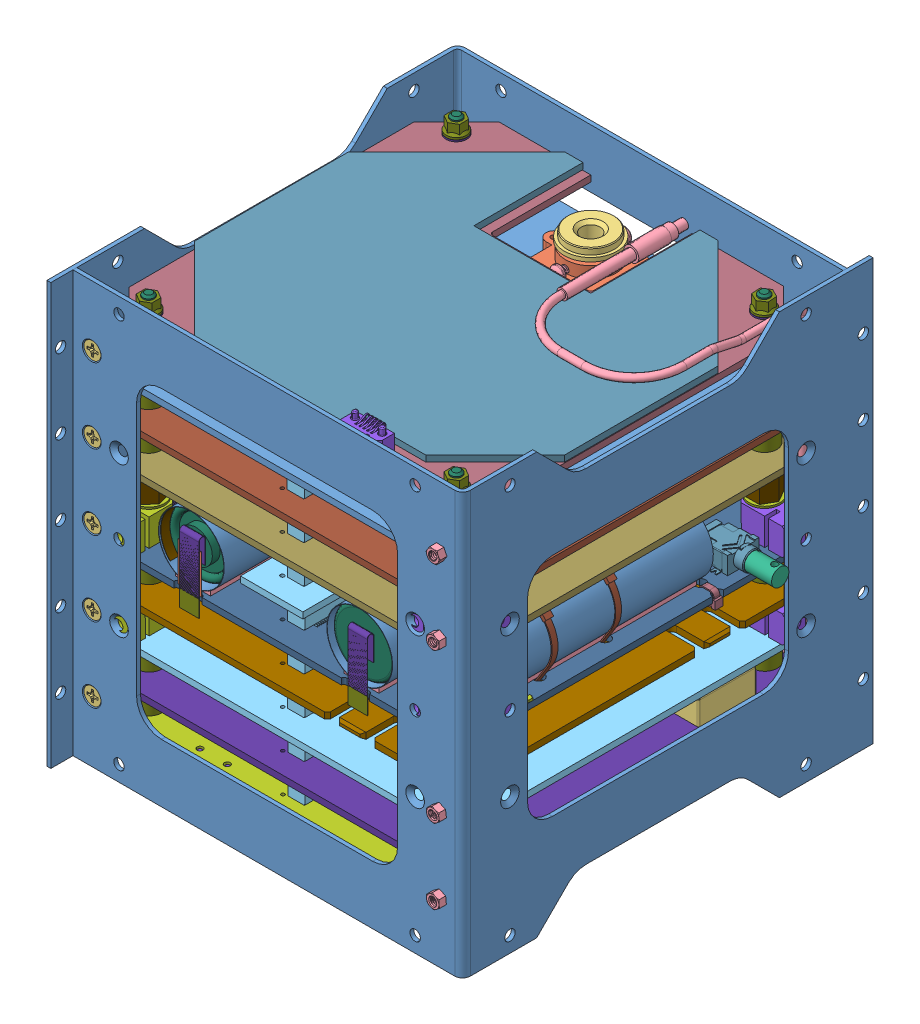
SolidWorks assembly FOX_FrameAssembly, configuration Default. Lengths in mm.
Overall size (104.5 108 111.03).
292 component instances, 63 part files, 95 mates.
Components (placement in the parent):
- FOX_ME_111_Walls-1: FOX_ME_111_Walls [Default] at (75.0611 9.8692 29.0204) size (100.17 108 105.36)
- FOX_ME_111_Walls-2: FOX_ME_111_Walls [Default] at (-24.2839 9.8692 -70.6584) x (-1 0 0) z (0 0 -1) size (100.17 108 105.36)
- 90945A705_18-8 Stainless Steel Mil. Spec. Washer-1: 90945A705_18-8 Stainless Steel Mil. Spec. Washer [90945A705] at (70.0611 -28.5308 28.0204) x (1 0 0) z (0 -1 0) size (3.78 0.46 3.78)
- 90945A705_18-8 Stainless Steel Mil. Spec. Washer-2: 90945A705_18-8 Stainless Steel Mil. Spec. Washer [90945A705] at (-19.2839 -28.5308 -69.6584) x (1 0 0) z (0 1 0) size (3.78 0.46 3.78)
- 90945A705_18-8 Stainless Steel Mil. Spec. Washer-3: 90945A705_18-8 Stainless Steel Mil. Spec. Washer [90945A705] at (-19.2839 29.0692 -69.6584) x (1 0 0) z (0 1 0) size (3.78 0.46 3.78)
- 90945A705_18-8 Stainless Steel Mil. Spec. Washer-4: 90945A705_18-8 Stainless Steel Mil. Spec. Washer [90945A705] at (-19.2839 -9.3308 -69.6584) x (1 0 0) z (0 1 0) size (3.78 0.46 3.78)
- 90945A705_18-8 Stainless Steel Mil. Spec. Washer-5: 90945A705_18-8 Stainless Steel Mil. Spec. Washer [90945A705] at (70.0611 9.8692 -68.6584) x (1 0 0) z (0 -1 0) size (3.78 0.46 3.78)
- 90945A705_18-8 Stainless Steel Mil. Spec. Washer-6: 90945A705_18-8 Stainless Steel Mil. Spec. Washer [90945A705] at (-19.2839 9.8692 -69.6584) x (1 0 0) z (0 1 0) size (3.78 0.46 3.78)
- 90945A705_18-8 Stainless Steel Mil. Spec. Washer-7: 90945A705_18-8 Stainless Steel Mil. Spec. Washer [90945A705] at (70.0611 -9.3308 28.0204) x (1 0 0) z (0 -1 0) size (3.78 0.46 3.78)
- 90945A705_18-8 Stainless Steel Mil. Spec. Washer-8: 90945A705_18-8 Stainless Steel Mil. Spec. Washer [90945A705] at (70.0611 48.2692 28.0204) x (1 0 0) z (0 -1 0) size (3.78 0.46 3.78)
- 90945A705_18-8 Stainless Steel Mil. Spec. Washer-9: 90945A705_18-8 Stainless Steel Mil. Spec. Washer [90945A705] at (70.0611 29.0692 28.0204) x (1 0 0) z (0 -1 0) size (3.78 0.46 3.78)
- 90945A705_18-8 Stainless Steel Mil. Spec. Washer-20: 90945A705_18-8 Stainless Steel Mil. Spec. Washer [90945A705] at (-19.2839 48.2692 -70.1156) x (1 0 0) z (0 -1 0) size (3.78 0.46 3.78)
- 93085A017_Mil. Spec. Stainless Steel Phillips Flat Head Screws-1: 93085A017_Mil. Spec. Stainless Steel Phillips Flat Head Screws [93085A017] at (-19.2839 9.8692 25.6645) size (4.37 4.37 6.55)
- 93085A017_Mil. Spec. Stainless Steel Phillips Flat Head Screws-2: 93085A017_Mil. Spec. Stainless Steel Phillips Flat Head Screws [93085A017] at (-19.2839 48.2692 25.6645) size (4.37 4.37 6.55)
- 93085A017_Mil. Spec. Stainless Steel Phillips Flat Head Screws-3: 93085A017_Mil. Spec. Stainless Steel Phillips Flat Head Screws [93085A017] at (-19.2839 -9.3308 25.6645) size (4.37 4.37 6.55)
- 93085A017_Mil. Spec. Stainless Steel Phillips Flat Head Screws-4: 93085A017_Mil. Spec. Stainless Steel Phillips Flat Head Screws [93085A017] at (-19.2839 -28.5308 25.6645) size (4.37 4.37 6.55)
- 93085A017_Mil. Spec. Stainless Steel Phillips Flat Head Screws-5: 93085A017_Mil. Spec. Stainless Steel Phillips Flat Head Screws [93085A017] at (-19.2839 29.0692 25.6645) size (4.37 4.37 6.55)
- 93085A017_Mil. Spec. Stainless Steel Phillips Flat Head Screws-6: 93085A017_Mil. Spec. Stainless Steel Phillips Flat Head Screws [93085A017] at (70.0611 -28.5308 -67.3025) x (1 0 0) z (0 0 -1) size (4.37 4.37 6.55)
- 93085A017_Mil. Spec. Stainless Steel Phillips Flat Head Screws-7: 93085A017_Mil. Spec. Stainless Steel Phillips Flat Head Screws [93085A017] at (70.0611 -9.3308 -67.3025) x (1 0 0) z (0 0 -1) size (4.37 4.37 6.55)
- 93085A017_Mil. Spec. Stainless Steel Phillips Flat Head Screws-8: 93085A017_Mil. Spec. Stainless Steel Phillips Flat Head Screws [93085A017] at (70.0611 9.8692 -67.3025) x (1 0 0) z (0 0 -1) size (4.37 4.37 6.55)
- 93085A017_Mil. Spec. Stainless Steel Phillips Flat Head Screws-9: 93085A017_Mil. Spec. Stainless Steel Phillips Flat Head Screws [93085A017] at (70.0611 29.0692 -67.3025) x (1 0 0) z (0 0 -1) size (4.37 4.37 6.55)
- 93085A017_Mil. Spec. Stainless Steel Phillips Flat Head Screws-10: 93085A017_Mil. Spec. Stainless Steel Phillips Flat Head Screws [93085A017] at (70.0611 48.2692 -67.3025) x (-1 0 0) z (0 0 -1) size (4.37 4.37 6.55)
- 95307A800_Mil. Spec. Distorted-Thread Flange Locknut-1: 95307A800_Mil. Spec. Distorted-Thread Flange Locknut [95307A800] at (70.0611 -9.3308 29.6682) x (0.377464 0.926024 0) z (0 0 1) size (4.24 4.24 2.44)
- 95307A800_Mil. Spec. Distorted-Thread Flange Locknut-2: 95307A800_Mil. Spec. Distorted-Thread Flange Locknut [95307A800] at (70.0611 48.2692 29.6682) x (-0.835302 0.549792 0) z (0 0 1) size (4.24 4.24 2.44)
- 95307A800_Mil. Spec. Distorted-Thread Flange Locknut-3: 95307A800_Mil. Spec. Distorted-Thread Flange Locknut [95307A800] at (70.0611 29.0692 29.6682) x (0.533227 -0.845972 0) z (0 0 1) size (4.24 4.24 2.44)
- 95307A800_Mil. Spec. Distorted-Thread Flange Locknut-4: 95307A800_Mil. Spec. Distorted-Thread Flange Locknut [95307A800] at (70.0611 9.8692 -67.0106) x (-0.854944 -0.518721 0) z (0 0 1) size (4.24 4.24 2.44)
- 95307A800_Mil. Spec. Distorted-Thread Flange Locknut-5: 95307A800_Mil. Spec. Distorted-Thread Flange Locknut [95307A800] at (70.0611 -28.5308 29.6682) x (0.994964 0.100237 0) z (0 0 1) size (4.24 4.24 2.44)
- 95307A800_Mil. Spec. Distorted-Thread Flange Locknut-6: 95307A800_Mil. Spec. Distorted-Thread Flange Locknut [95307A800] at (-19.2839 48.2692 -71.3063) x (-0.82039 0.571804 0) z (0 0 -1) size (4.24 4.24 2.44)
- 95307A800_Mil. Spec. Distorted-Thread Flange Locknut-7: 95307A800_Mil. Spec. Distorted-Thread Flange Locknut [95307A800] at (-19.2839 29.0692 -71.3063) x (-0.204746 -0.978815 0) z (0 0 -1) size (4.24 4.24 2.44)
- 95307A800_Mil. Spec. Distorted-Thread Flange Locknut-8: 95307A800_Mil. Spec. Distorted-Thread Flange Locknut [95307A800] at (-19.2839 9.8692 -71.3063) x (0.176402 -0.984318 0) z (0 0 -1) size (4.24 4.24 2.44)
- 95307A800_Mil. Spec. Distorted-Thread Flange Locknut-9: 95307A800_Mil. Spec. Distorted-Thread Flange Locknut [95307A800] at (-19.2839 -9.3308 -71.3063) x (-0.547588 0.836748 0) z (0 0 -1) size (4.24 4.24 2.44)
- 95307A800_Mil. Spec. Distorted-Thread Flange Locknut-10: 95307A800_Mil. Spec. Distorted-Thread Flange Locknut [95307A800] at (-19.2839 -28.5308 -71.3063) x (0.98812 0.153685 0) z (0 0 -1) size (4.24 4.24 2.44)
- PCB-Stack-1: PCB-Stack [Default] at (24.8941 -34.8331 -20.5973) x (1 0 0) z (0 0.999997 0.002368) size (103.5 98 104.43)
  - PCB-Stack.iam-1: PCB-Stack.iam [Default] at origin size (103.5 98 104.43)
    - PCB_TX.iam-1: PCB_TX.iam [Default] at origin size (95 95 16.51)
      - Samtec_QTH-030-02-L-D-A.ipt-1: Samtec_QTH-030-02-L-D-A.ipt [Default] at (0 -31.9938 1.8415) x (0 1 0) z (1 0 0) size (20 8 7.11)
      - Samtec_QSH-030-01-L-D-A.ipt-1: Samtec_QSH-030-01-L-D-A.ipt [Default] at (0 -31.9936 -0.127) x (0 -1 0) z (1 0 0) size (21.31 4 7.49)
      - PCB_TX.ipt-1: PCB_TX.ipt [Default] at origin size (95 95 1.59)
      - Samtec_FSI-105-06-L-S-AD.ipt-1: Samtec_FSI-105-06-L-S-AD.ipt [Default] at (-15 -42.5 -0.2) x (1 0 0) z (0 1 0) size (10 8.86 5.87)
      - C&K_HDT0004.iam-1: C&K_HDT0004.iam [Default] at (44.25 -44.5 0) x (1 0 0) z (0 1 0) size (4.99 3.82 4.7)
        - C&K_HDT0004.ipt-1: C&K_HDT0004.ipt [Default] at origin size (4.9 2.3 4.7)
        - C&K_HDT0004_blade.ipt-1: C&K_HDT0004_blade.ipt [Default] at (0.0272 0.0212 0) x (0.999834 0.018233 0) z (0 0 1) size (2.26 1.67 0.7)
        - C&K_HDT0004_blade.ipt-2: C&K_HDT0004_blade.ipt [Default] at (-0.9606 -0.3806 0) x (0.850594 -0.525824 0) z (0 0 1) size (2.26 1.67 0.7)
      - C&K_HDT0004.iam-2: C&K_HDT0004.iam [Default] at (-44.25 44.5 0) x (-1 0 0) z (0 -1 0) size (4.99 3.82 4.7)
        - C&K_HDT0004.ipt-1: C&K_HDT0004.ipt [Default] at origin size (4.9 2.3 4.7)
        - C&K_HDT0004_blade.ipt-1: C&K_HDT0004_blade.ipt [Default] at (0.0272 0.0212 0) x (0.999834 0.018233 0) z (0 0 1) size (2.26 1.67 0.7)
        - C&K_HDT0004_blade.ipt-2: C&K_HDT0004_blade.ipt [Default] at (-0.9606 -0.3806 0) x (0.850594 -0.525824 0) z (0 0 1) size (2.26 1.67 0.7)
      - Tantalum_4x9x1.ipt-1: Tantalum_4x9x1.ipt [Default] at (10.5 -13.5 3.8375) x (0 1 0) z (0 0 1) size (8.75 4 1)
      - Tantalum_5x7x1.ipt-1: Tantalum_5x7x1.ipt [Default] at (-24 20.25 4.0875) x (-1 0 0) z (0 0 1) size (7 5 1)
      - tx_v2_04_cu_shield.ipt-1: tx_v2_04_cu_shield.ipt [Default] at (-0.2089 -0.202 7.5561) size (77.88 35.38 7.85)
      - Pb_TX_bot.ipt-1: Pb_TX_bot.ipt [Default] at (0 0 -0.9874) size (95 82 1.57)
      - coax_tx.ipt-1: coax_tx.ipt [Default] at (42 22.5 -0.9) x (-1 0 0) z (0 0 -1) size (40.9 68.4 4.41)
    - standoff815mm.ipt-1: standoff815mm.ipt [Default] at (-39.5 -39.5 5.6625) size (6.35 6.35 8.15)
    - standoff815mm.ipt-2: standoff815mm.ipt [Default] at (-39.5 39.5 5.6625) size (6.35 6.35 8.15)
    - standoff815mm.ipt-3: standoff815mm.ipt [Default] at (39.5 39.5 5.6625) size (6.35 6.35 8.15)
    - standoff815mm.ipt-4: standoff815mm.ipt [Default] at (39.5 -39.5 5.6625) size (6.35 6.35 8.15)
    - standoff815mm.ipt-5: standoff815mm.ipt [Default] at (-39.5 -39.5 15.4) size (6.35 6.35 8.15)
    - standoff815mm.ipt-6: standoff815mm.ipt [Default] at (-39.5 39.5 15.4) size (6.35 6.35 8.15)
    - standoff815mm.ipt-7: standoff815mm.ipt [Default] at (39.5 39.5 15.4) size (6.35 6.35 8.15)
    - standoff815mm.ipt-8: standoff815mm.ipt [Default] at (39.5 -39.5 15.4) size (6.35 6.35 8.15)
    - standoff815mm.ipt-9: standoff815mm.ipt [Default] at (-39.5 39.5 25.1375) size (6.35 6.35 8.15)
    - standoff815mm.ipt-10: standoff815mm.ipt [Default] at (39.5 -39.5 25.1375) size (6.35 6.35 8.15)
    - standoff815mm.ipt-11: standoff815mm.ipt [Default] at (-39.5 -39.5 34.875) size (6.35 6.35 8.15)
    - standoff815mm.ipt-12: standoff815mm.ipt [Default] at (-39.5 39.5 34.875) size (6.35 6.35 8.15)
    - standoff815mm.ipt-13: standoff815mm.ipt [Default] at (39.5 39.5 34.875) size (6.35 6.35 8.15)
    - standoff815mm.ipt-14: standoff815mm.ipt [Default] at (39.5 -39.5 34.875) size (6.35 6.35 8.15)
    - standoff815mm.ipt-15: standoff815mm.ipt [Default] at (-39.5 -39.5 64.0875) size (6.35 6.35 8.15)
    - standoff815mm.ipt-16: standoff815mm.ipt [Default] at (39.5 39.5 64.0875) size (6.35 6.35 8.15)
    - standoff815mm.ipt-17: standoff815mm.ipt [Default] at (-39.5 -39.5 73.825) size (6.35 6.35 8.15)
    - standoff815mm.ipt-18: standoff815mm.ipt [Default] at (-39.5 39.5 73.825) size (6.35 6.35 8.15)
    - standoff815mm.ipt-19: standoff815mm.ipt [Default] at (39.5 39.5 73.825) size (6.35 6.35 8.15)
    - standoff815mm.ipt-20: standoff815mm.ipt [Default] at (39.5 -39.5 73.825) size (6.35 6.35 8.15)
    - standoff815mm.ipt-21: standoff815mm.ipt [Default] at (-39.5 -39.5 83.5625) size (6.35 6.35 8.15)
    - standoff815mm.ipt-22: standoff815mm.ipt [Default] at (-39.5 39.5 83.5625) size (6.35 6.35 8.15)
    - standoff815mm.ipt-23: standoff815mm.ipt [Default] at (39.5 39.5 83.5625) size (6.35 6.35 8.15)
    - standoff815mm.ipt-24: standoff815mm.ipt [Default] at (39.5 -39.5 83.5625) size (6.35 6.35 8.15)
    - PCB_RX.iam-1: PCB_RX.iam [Default] at (0 0 9.7375) size (95 95 87.7)
      - Samtec_QSH-030-01-L-D-A.ipt-1: Samtec_QSH-030-01-L-D-A.ipt [Default] at (0 -31.9936 -0.127) x (0 -1 0) z (1 0 0) size (21.31 4 7.49)
      - Samtec_QTH-030-02-L-D-A.ipt-1: Samtec_QTH-030-02-L-D-A.ipt [Default] at (0 -31.9938 1.8415) x (0 1 0) z (1 0 0) size (20 8 7.11)
      - PCB_RX.ipt-1: PCB_RX.ipt [Default] at origin size (95 95 1.59)
      - RX_tan_U7_MBC13917.ipt-1: RX_tan_U7_MBC13917.ipt [Default] at (4.5 42.03 -1) x (-1 0 0) z (0 0 1) size (6.35 6.35 1)
      - RX_tan_U9_SA601.ipt-1: RX_tan_U9_SA601.ipt [Default] at (-23.16 37.32 -1) x (-1 0 0) z (0 0 1) size (6.35 6.35 1)
      - RX_tan_U10_SA607.ipt-1: RX_tan_U10_SA607.ipt [Default] at (-18 4 -1) x (-1 0 0) z (0 0 1) size (6.35 6.35 1)
      - rx_v1_23_cu_shield.ipt-1: rx_v1_23_cu_shield.ipt [Default] at (0 0 7.5565) size (91.38 65.38 7.85)
      - rx_coax.ipt-1: rx_coax.ipt [Default] at (25.5 41.6 2.6035) x (1 0 0) z (0 -1 0) size (34.34 82.88 45.77)
    - PCB_IHU.iam-1: PCB_IHU.iam [Default] at (0 0 19.475) size (95 95 12.08)
      - Samtec_QSH-030-01-L-D-A.ipt-1: Samtec_QSH-030-01-L-D-A.ipt [Default] at (0 -31.9936 -0.127) x (0 -1 0) z (1 0 0) size (21.31 4 7.49)
      - Samtec_QTH-030-02-L-D-A.ipt-1: Samtec_QTH-030-02-L-D-A.ipt [Default] at (0 -31.9938 1.8415) x (0 1 0) z (1 0 0) size (20 8 7.11)
      - PCB_IHU.ipt-1: PCB_IHU.ipt [Default] at origin size (95 95 1.59)
    - spacer_copper.ipt-1: spacer_copper.ipt [Default] at (-39.5 -39.5 25.1375) size (4.76 4.76 8.15)
    - spacer_copper.ipt-2: spacer_copper.ipt [Default] at (39.5 39.5 25.1375) size (4.76 4.76 8.15)
    - spacer_copper.ipt-3: spacer_copper.ipt [Default] at (-39.5 -39.5 44.6125) size (4.76 4.76 8.15)
    - spacer_copper.ipt-4: spacer_copper.ipt [Default] at (-39.5 39.5 44.6125) size (4.76 4.76 8.15)
    - spacer_copper.ipt-5: spacer_copper.ipt [Default] at (39.5 39.5 44.6125) size (4.76 4.76 8.15)
    - spacer_copper.ipt-6: spacer_copper.ipt [Default] at (39.5 -39.5 44.6125) size (4.76 4.76 8.15)
    - spacer_copper.ipt-7: spacer_copper.ipt [Default] at (39.5 -39.5 55.9375) x (0.997727 -0.067389 0) z (0 0 -1) size (4.76 4.76 8.15)
    - spacer_copper.ipt-8: spacer_copper.ipt [Default] at (-39.5 39.5 55.9375) x (1 0 0) z (0 0 -1) size (4.76 4.76 8.15)
    - 90792A312_shimwasher.ipt-1: 90792A312_shimwasher.ipt [Default] at (-39.5 -39.5 21.0625) size (7.95 7.95 0.25)
    - 90792A312_shimwasher.ipt-2: 90792A312_shimwasher.ipt [Default] at (39.5 39.5 21.0625) size (7.95 7.95 0.25)
    - 90792A312_shimwasher.ipt-3: 90792A312_shimwasher.ipt [Default] at (-39.5 -39.5 28.6375) size (7.95 7.95 0.25)
    - 90792A312_shimwasher.ipt-4: 90792A312_shimwasher.ipt [Default] at (39.5 39.5 28.6375) size (7.95 7.95 0.25)
    - 90792A312_shimwasher.ipt-5: 90792A312_shimwasher.ipt [Default] at (-39.5 -39.5 40.5375) size (7.95 7.95 0.25)
    - 90792A312_shimwasher.ipt-6: 90792A312_shimwasher.ipt [Default] at (-39.5 -39.5 48.1125) size (7.95 7.95 0.25)
    - 90792A312_shimwasher.ipt-7: 90792A312_shimwasher.ipt [Default] at (-39.5 39.5 40.5375) size (7.95 7.95 0.25)
    - 90792A312_shimwasher.ipt-8: 90792A312_shimwasher.ipt [Default] at (-39.5 39.5 48.1125) size (7.95 7.95 0.25)
    - 90792A312_shimwasher.ipt-9: 90792A312_shimwasher.ipt [Default] at (39.5 39.5 40.5375) size (7.95 7.95 0.25)
    - 90792A312_shimwasher.ipt-10: 90792A312_shimwasher.ipt [Default] at (39.5 39.5 48.1125) size (7.95 7.95 0.25)
    - 90792A312_shimwasher.ipt-11: 90792A312_shimwasher.ipt [Default] at (39.5 -39.5 40.5375) size (7.95 7.95 0.25)
    - 90792A312_shimwasher.ipt-12: 90792A312_shimwasher.ipt [Default] at (39.5 -39.5 48.1125) size (7.95 7.95 0.25)
    - 90792A312_shimwasher.ipt-13: 90792A312_shimwasher.ipt [Default] at (-39.5 39.5 60.0125) size (7.95 7.95 0.25)
    - 90792A312_shimwasher.ipt-14: 90792A312_shimwasher.ipt [Default] at (-39.5 39.5 60.2665) size (7.95 7.95 0.25)
    - 90792A312_shimwasher.ipt-15: 90792A312_shimwasher.ipt [Default] at (39.5 -39.5 60.0125) size (7.95 7.95 0.25)
    - 90792A312_shimwasher.ipt-16: 90792A312_shimwasher.ipt [Default] at (39.5 -39.5 60.2665) size (7.95 7.95 0.25)
    - 90792A312_shimwasher.ipt-17: 90792A312_shimwasher.ipt [Default] at (-39.5 39.5 67.5205) size (7.95 7.95 0.25)
    - 90792A312_shimwasher.ipt-18: 90792A312_shimwasher.ipt [Default] at (-39.5 39.5 67.7745) size (7.95 7.95 0.25)
    - 90792A312_shimwasher.ipt-19: 90792A312_shimwasher.ipt [Default] at (39.5 -39.5 67.5205) size (7.95 7.95 0.25)
    - 90792A312_shimwasher.ipt-20: 90792A312_shimwasher.ipt [Default] at (39.5 -39.5 67.7745) size (7.95 7.95 0.25)
    - 90792A312_shimwasher.ipt-21: 90792A312_shimwasher.ipt [Default] at (-39.5 -39.5 21.3165) size (7.95 7.95 0.25)
    - 90792A312_shimwasher.ipt-22: 90792A312_shimwasher.ipt [Default] at (39.5 39.5 21.3165) size (7.95 7.95 0.25)
    - 90792A312_shimwasher.ipt-23: 90792A312_shimwasher.ipt [Default] at (-39.5 -39.5 28.8915) size (7.95 7.95 0.25)
    - 90792A312_shimwasher.ipt-24: 90792A312_shimwasher.ipt [Default] at (39.5 39.5 28.8915) size (7.95 7.95 0.25)
    - 90792A312_shimwasher.ipt-25: 90792A312_shimwasher.ipt [Default] at (39.5 -39.5 40.7915) size (7.95 7.95 0.25)
    - 90792A312_shimwasher.ipt-26: 90792A312_shimwasher.ipt [Default] at (-39.5 -39.5 40.7915) size (7.95 7.95 0.25)
    - 90792A312_shimwasher.ipt-27: 90792A312_shimwasher.ipt [Default] at (39.5 39.5 40.7915) size (7.95 7.95 0.25)
    - 90792A312_shimwasher.ipt-28: 90792A312_shimwasher.ipt [Default] at (-39.5 39.5 40.7915) size (7.95 7.95 0.25)
    - 90792A312_shimwasher.ipt-29: 90792A312_shimwasher.ipt [Default] at (-39.5 39.5 48.3665) size (7.95 7.95 0.25)
    - 90792A312_shimwasher.ipt-30: 90792A312_shimwasher.ipt [Default] at (-39.5 -39.5 48.3665) size (7.95 7.95 0.25)
    - 90792A312_shimwasher.ipt-31: 90792A312_shimwasher.ipt [Default] at (39.5 -39.5 48.3665) size (7.95 7.95 0.25)
    - 90792A312_shimwasher.ipt-32: 90792A312_shimwasher.ipt [Default] at (39.5 39.5 48.3665) size (7.95 7.95 0.25)
    - delrin_pcb_mount4.ipt-1: delrin_pcb_mount4.ipt [Default] at (49 49 25.1375) x (-1 0 0) z (0 0 1) size (14 14 7)
    - delrin_pcb_mount4.ipt-2: delrin_pcb_mount4.ipt [Default] at (-49 49 44.6125) x (0 -1 0) z (0 0 1) size (14 14 7)
    - delrin_pcb_mount4.ipt-3: delrin_pcb_mount4.ipt [Default] at (49 49 44.6125) x (-1 0 0) z (0 0 1) size (14 14 7)
    - delrin_pcb_mount4.ipt-4: delrin_pcb_mount4.ipt [Default] at (49 -49 44.6125) x (0 1 0) z (0 0 1) size (14 14 7)
    - delrin_pcb_mount4.ipt-5: delrin_pcb_mount4.ipt [Default] at (-49 49 64.0205) x (0 -1 0) z (0 0 1) size (14 14 7)
    - delrin_pcb_mount4.ipt-6: delrin_pcb_mount4.ipt [Default] at (49 -49 64.0205) x (0 1 0) z (0 0 1) size (14 14 7)
    - PCB_PSU.iam-1: PCB_PSU.iam [Default] at (0 0 29.2125) size (95 95 12.08)
      - Samtec_QSH-030-01-L-D-A.ipt-1: Samtec_QSH-030-01-L-D-A.ipt [Default] at (0 -31.9936 -0.127) x (0 -1 0) z (1 0 0) size (21.31 4 7.49)
      - Samtec_QTH-030-02-L-D-A.ipt-1: Samtec_QTH-030-02-L-D-A.ipt [Default] at (0 -31.9938 1.8415) x (0 1 0) z (1 0 0) size (20 8 7.11)
      - PCB_PSU.ipt-1: PCB_PSU.ipt [Default] at origin size (95 95 1.59)
    - battery6A.iam-1: battery6A.iam [Default] at (0 0 44.5375) size (95.25 95.25 22.75)
      - PCB_Batt1.iam-1: PCB_Batt1.iam [Default] at (0 0 -5.5875) size (95 95 12.08)
        - PCB_Batt1.ipt-1: PCB_Batt1.ipt [Default] at origin size (95 95 1.59)
        - Samtec_QSH-030-01-L-D-A.ipt-1: Samtec_QSH-030-01-L-D-A.ipt [Default] at (0 -31.9936 -0.127) x (0 -1 0) z (1 0 0) size (21.31 4 7.49)
        - Samtec_QTH-030-02-L-D-A.ipt-1: Samtec_QTH-030-02-L-D-A.ipt [Default] at (0 -31.9938 1.8415) x (0 1 0) z (1 0 0) size (20 8 7.11)
      - battery_cord_2x.ipt-1: battery_cord_2x.ipt [Default] at (30.1001 -22 -5.95) x (0 1 0) z (1 0 0) size (2 19.3 34.3)
      - battery_cord_2x.ipt-2: battery_cord_2x.ipt [Default] at (30 -5.6143 -5.95) x (0 1 0) z (1 0 0) size (2 19.3 34.3)
      - battery_cord_2x.ipt-3: battery_cord_2x.ipt [Default] at (-30.1001 -22 -5.95) x (0 -1 0) z (-1 0 0) size (2 19.3 34.3)
      - battery_cord_2x.ipt-4: battery_cord_2x.ipt [Default] at (-30 -5.6143 -5.95) x (0 -1 0) z (-1 0 0) size (2 19.3 34.3)
      - battery_cord_2x.ipt-5: battery_cord_2x.ipt [Default] at (15.5 30.1001 -5.95) x (-1 0 0) z (0 1 0) size (2 19.3 34.3)
      - battery_cord_2x.ipt-6: battery_cord_2x.ipt [Default] at (-15.5 30.1001 -5.95) x (-1 0 0) z (0 1 0) size (2 19.3 34.3)
      - hysteresis_rod.ipt-1: hysteresis_rod.ipt [Default] at (45.25 0 -6.4003) x (0 0 1) z (0 1 0) size (1.57 1.57 76.2)
      - hysteresis_rod.ipt-2: hysteresis_rod.ipt [Default] at (0 45.25 -6.4003) x (0 0 1) z (-1 0 0) size (1.57 1.57 76.2)
      - hysteresis_cord.ipt-1: hysteresis_cord.ipt [Default] at (45.25 -33.45 -3.85) x (0 -1 0) z (1 0 0) size (2 3.9 4.45)
      - hysteresis_cord.ipt-2: hysteresis_cord.ipt [Default] at (45.25 19.55 -3.85) x (0 -1 0) z (1 0 0) size (2 3.9 4.45)
      - hysteresis_cord.ipt-3: hysteresis_cord.ipt [Default] at (27 45.25 -3.85) x (1 0 0) z (0 1 0) size (2 3.9 4.45)
      - hysteresis_cord.ipt-4: hysteresis_cord.ipt [Default] at (-27 45.25 -3.85) x (1 0 0) z (0 1 0) size (2 3.9 4.45)
      - CUI_audio_SJ1-42536-SMT.ipt-1: CUI_audio_SJ1-42536-SMT.ipt [Default] at (45 28.5 -1.42) x (1 0 0) z (0 -1 0) size (12.5 5.6 10.4)
      - battery_A_SanyoKR1700AU.iam-1: battery_A_SanyoKR1700AU.iam [Default] at (-38.5 -6.5 4.45) x (0 0 1) z (0 -1 0) size (22.45 16.9 51.9)
        - battery_A_SanyoKR1700AU.ipt-1: battery_A_SanyoKR1700AU.ipt [Default] at origin size (16.5 16.5 48.5)
        - battery_tab_straight.ipt-1: battery_tab_straight.ipt [Default] at (0 0 -24.35) x (0 0 -1) z (0 -1 0) size (1.7 17.85 5)
        - battery_tab_straight.ipt-2: battery_tab_straight.ipt [Default] at (0 0 24.35) x (0 0 1) z (0 1 0) size (1.7 17.85 5)
        - battery_tab_folded.ipt-1: battery_tab_folded.ipt [Default] at (0 0 -24.35) x (0 0 -1) z (0 -1 0) size (3.6 14.15 5)
        - battery_tab_folded.ipt-2: battery_tab_folded.ipt [Default] at (0 0 24.35) x (0 0 1) z (0 1 0) size (3.6 14.15 5)
        - kaptonheater_OmegaKHLV102.ipt-1: kaptonheater_OmegaKHLV102.ipt [Default] at origin size (14.25 14.25 50)
        - kapton_wrap_battery.ipt-1: kapton_wrap_battery.ipt [Default] at origin size (16.9 16.9 50.8)
        - kapton_battery_tab.ipt-1: kapton_battery_tab.ipt [Default] at (-4 0 25.75) x (0 -1 0) z (0 0 1) size (6 10 0.1)
      - battery_A_SanyoKR1700AU.iam-2: battery_A_SanyoKR1700AU.iam [Default] at (-21.6 -21.1143 4.45) x (0 0 1) z (0 -1 0) size (22.45 16.9 51.9)
        - battery_A_SanyoKR1700AU.ipt-1: battery_A_SanyoKR1700AU.ipt [Default] at origin size (16.5 16.5 48.5)
        - battery_tab_straight.ipt-1: battery_tab_straight.ipt [Default] at (0 0 -24.35) x (0 0 -1) z (0 -1 0) size (1.7 17.85 5)
        - battery_tab_straight.ipt-2: battery_tab_straight.ipt [Default] at (0 0 24.35) x (0 0 1) z (0 1 0) size (1.7 17.85 5)
        - battery_tab_folded.ipt-1: battery_tab_folded.ipt [Default] at (0 0 -24.35) x (0 0 -1) z (0 -1 0) size (3.6 14.15 5)
        - battery_tab_folded.ipt-2: battery_tab_folded.ipt [Default] at (0 0 24.35) x (0 0 1) z (0 1 0) size (3.6 14.15 5)
        - kaptonheater_OmegaKHLV102.ipt-1: kaptonheater_OmegaKHLV102.ipt [Default] at origin size (14.25 14.25 50)
        - kapton_wrap_battery.ipt-1: kapton_wrap_battery.ipt [Default] at origin size (16.9 16.9 50.8)
        - kapton_battery_tab.ipt-1: kapton_battery_tab.ipt [Default] at (-4 0 25.75) x (0 -1 0) z (0 0 1) size (6 10 0.1)
      - battery_A_SanyoKR1700AU.iam-3: battery_A_SanyoKR1700AU.iam [Default] at (0 38.5 4.45) x (0 0 1) z (-1 0 0) size (22.45 16.9 51.9)
        - battery_A_SanyoKR1700AU.ipt-1: battery_A_SanyoKR1700AU.ipt [Default] at origin size (16.5 16.5 48.5)
        - battery_tab_straight.ipt-1: battery_tab_straight.ipt [Default] at (0 0 -24.35) x (0 0 -1) z (0 -1 0) size (1.7 17.85 5)
        - battery_tab_straight.ipt-2: battery_tab_straight.ipt [Default] at (0 0 24.35) x (0 0 1) z (0 1 0) size (1.7 17.85 5)
        - battery_tab_folded.ipt-1: battery_tab_folded.ipt [Default] at (0 0 -24.35) x (0 0 -1) z (0 -1 0) size (3.6 14.15 5)
        - battery_tab_folded.ipt-2: battery_tab_folded.ipt [Default] at (0 0 24.35) x (0 0 1) z (0 1 0) size (3.6 14.15 5)
        - kaptonheater_OmegaKHLV102.ipt-1: kaptonheater_OmegaKHLV102.ipt [Default] at origin size (14.25 14.25 50)
        - kapton_wrap_battery.ipt-1: kapton_wrap_battery.ipt [Default] at origin size (16.9 16.9 50.8)
        - kapton_battery_tab.ipt-1: kapton_battery_tab.ipt [Default] at (-4 0 25.75) x (0 -1 0) z (0 0 1) size (6 10 0.1)
      - battery_A_SanyoKR1700AU.iam-4: battery_A_SanyoKR1700AU.iam [Default] at (0 21.6 4.45) x (0 0 1) z (-1 0 0) size (22.45 16.9 51.9)
        - battery_A_SanyoKR1700AU.ipt-1: battery_A_SanyoKR1700AU.ipt [Default] at origin size (16.5 16.5 48.5)
        - battery_tab_straight.ipt-1: battery_tab_straight.ipt [Default] at (0 0 -24.35) x (0 0 -1) z (0 -1 0) size (1.7 17.85 5)
        - battery_tab_straight.ipt-2: battery_tab_straight.ipt [Default] at (0 0 24.35) x (0 0 1) z (0 1 0) size (1.7 17.85 5)
        - battery_tab_folded.ipt-1: battery_tab_folded.ipt [Default] at (0 0 -24.35) x (0 0 -1) z (0 -1 0) size (3.6 14.15 5)
        - battery_tab_folded.ipt-2: battery_tab_folded.ipt [Default] at (0 0 24.35) x (0 0 1) z (0 1 0) size (3.6 14.15 5)
        - kaptonheater_OmegaKHLV102.ipt-1: kaptonheater_OmegaKHLV102.ipt [Default] at origin size (14.25 14.25 50)
        - kapton_wrap_battery.ipt-1: kapton_wrap_battery.ipt [Default] at origin size (16.9 16.9 50.8)
        - kapton_battery_tab.ipt-1: kapton_battery_tab.ipt [Default] at (-4 0 25.75) x (0 -1 0) z (0 0 1) size (6 10 0.1)
      - battery_A_SanyoKR1700AU.iam-5: battery_A_SanyoKR1700AU.iam [Default] at (21.6 -21.1143 4.45) x (0 0 1) z (0 1 0) size (22.45 16.9 51.9)
        - battery_A_SanyoKR1700AU.ipt-1: battery_A_SanyoKR1700AU.ipt [Default] at origin size (16.5 16.5 48.5)
        - battery_tab_straight.ipt-1: battery_tab_straight.ipt [Default] at (0 0 -24.35) x (0 0 -1) z (0 -1 0) size (1.7 17.85 5)
        - battery_tab_straight.ipt-2: battery_tab_straight.ipt [Default] at (0 0 24.35) x (0 0 1) z (0 1 0) size (1.7 17.85 5)
        - battery_tab_folded.ipt-1: battery_tab_folded.ipt [Default] at (0 0 -24.35) x (0 0 -1) z (0 -1 0) size (3.6 14.15 5)
        - battery_tab_folded.ipt-2: battery_tab_folded.ipt [Default] at (0 0 24.35) x (0 0 1) z (0 1 0) size (3.6 14.15 5)
        - kaptonheater_OmegaKHLV102.ipt-1: kaptonheater_OmegaKHLV102.ipt [Default] at origin size (14.25 14.25 50)
        - kapton_wrap_battery.ipt-1: kapton_wrap_battery.ipt [Default] at origin size (16.9 16.9 50.8)
        - kapton_battery_tab.ipt-1: kapton_battery_tab.ipt [Default] at (-4 0 25.75) x (0 -1 0) z (0 0 1) size (6 10 0.1)
      - battery_A_SanyoKR1700AU.iam-6: battery_A_SanyoKR1700AU.iam [Default] at (38.5 -6.5 4.45) x (0 0 1) z (0 1 0) size (22.45 16.9 51.9)
        - battery_A_SanyoKR1700AU.ipt-1: battery_A_SanyoKR1700AU.ipt [Default] at origin size (16.5 16.5 48.5)
        - battery_tab_straight.ipt-1: battery_tab_straight.ipt [Default] at (0 0 -24.35) x (0 0 -1) z (0 -1 0) size (1.7 17.85 5)
        - battery_tab_straight.ipt-2: battery_tab_straight.ipt [Default] at (0 0 24.35) x (0 0 1) z (0 1 0) size (1.7 17.85 5)
        - battery_tab_folded.ipt-1: battery_tab_folded.ipt [Default] at (0 0 -24.35) x (0 0 -1) z (0 -1 0) size (3.6 14.15 5)
        - battery_tab_folded.ipt-2: battery_tab_folded.ipt [Default] at (0 0 24.35) x (0 0 1) z (0 1 0) size (3.6 14.15 5)
        - kaptonheater_OmegaKHLV102.ipt-1: kaptonheater_OmegaKHLV102.ipt [Default] at origin size (14.25 14.25 50)
        - kapton_wrap_battery.ipt-1: kapton_wrap_battery.ipt [Default] at origin size (16.9 16.9 50.8)
        - kapton_battery_tab.ipt-1: kapton_battery_tab.ipt [Default] at (-4 0 25.75) x (0 -1 0) z (0 0 1) size (6 10 0.1)
      - signal_relay_panasonic_tx.ipt-1: signal_relay_panasonic_tx.ipt [Default] at (4.5 3.5 0.1) x (1 0 0) z (0 -1 0) size (15 8.2 7.4)
      - signal_relay_panasonic_tx.ipt-2: signal_relay_panasonic_tx.ipt [Default] at (-8 -5 0.1) x (0 1 0) z (-1 0 0) size (15 8.2 7.4)
      - epoxy_under-battery.ipt-1: epoxy_under-battery.ipt [Default] at (-38.5 -6.5 -4) x (-1 0 0) z (0 1 0) size (9 1.35 50)
      - epoxy_under-battery.ipt-2: epoxy_under-battery.ipt [Default] at (-21.6 -21.1143 -4) x (1 0 0) z (0 -1 0) size (9 1.35 50)
      - epoxy_under-battery.ipt-3: epoxy_under-battery.ipt [Default] at (0 38.5 -4) x (0 -1 0) z (-1 0 0) size (9 1.35 50)
      - epoxy_under-battery.ipt-4: epoxy_under-battery.ipt [Default] at (0 21.6 -4) x (0 -1 0) z (-1 0 0) size (9 1.35 50)
      - epoxy_under-battery.ipt-5: epoxy_under-battery.ipt [Default] at (21.6 -21.1143 -4) x (-1 0 0) z (0 1 0) size (9 1.35 50)
      - epoxy_under-battery.ipt-6: epoxy_under-battery.ipt [Default] at (38.5 -6.5 -4) x (-1 0 0) z (0 1 0) size (9 1.35 50)
      - epoxy_under-battery.ipt-7: epoxy_under-battery.ipt [Default] at (0 30 4.45) x (0 0 -1) z (1 0 0) size (9 1.35 50)
      - epoxy_under-battery.ipt-8: epoxy_under-battery.ipt [Default] at (0 30.1 4.45) x (0 0 -1) z (-1 0 0) size (9 1.35 50)
      - epoxy_under-battery_short.ipt-1: epoxy_under-battery_short.ipt [Default] at (-30 -13.45 4.45) x (0 0 -1) z (0 1 0) size (9 1.35 34.4)
      - epoxy_under-battery_short.ipt-2: epoxy_under-battery_short.ipt [Default] at (-30.1 -14.0643 4.45) x (0 0 -1) z (0 -1 0) size (9 1.35 34.4)
      - epoxy_under-battery_short.ipt-3: epoxy_under-battery_short.ipt [Default] at (30.1 -14.1643 4.45) x (0 0 -1) z (0 1 0) size (9 1.35 34.4)
      - epoxy_under-battery_short.ipt-4: epoxy_under-battery_short.ipt [Default] at (30 -13.55 4.45) x (0 0 -1) z (0 -1 0) size (9 1.35 34.4)
      - thermistor_batteries.ipt-1: thermistor_batteries.ipt [Default] at (-30.05 -14.11 8.95) x (-1 0 0) z (0 -1 0) size (2.29 2.29 20.08)
      - thermistor_batteries.ipt-2: thermistor_batteries.ipt [Default] at (30 -14.21 8.95) x (-1 0 0) z (0 -1 0) size (2.29 2.29 20.08)
      - thermistor_batteries.ipt-3: thermistor_batteries.ipt [Default] at (0 30 8.95) x (0 -1 0) z (1 0 0) size (2.29 2.29 20.08)
      - LED_LTST-S270KFKT.ipt-1: LED_LTST-S270KFKT.ipt [Default] at (-46.35 -28.5 -3.7) size (1.15 1.65 0.6)
      - LED_LTST-S270KFKT.ipt-2: LED_LTST-S270KFKT.ipt [Default] at (46.35 -28.5 -3.7) x (-1 0 0) z (0 0 -1) size (1.15 1.65 0.6)
      - shielded_power_inductor_CC1360.ipt-1: shielded_power_inductor_CC1360.ipt [Default] at (6 -13.5 -3.1) x (0 -1 0) z (0 0 1) size (12.7 12.6 5.45)
      - piezo_sounder_PKLCS.ipt-1: piezo_sounder_PKLCS.ipt [Default] at (-7.5 -13.5 -2.5) x (0 1 0) z (0 0 1) size (12 12 3)
      - MiniUSB-B_Molex548190519.ipt-1: MiniUSB-B_Molex548190519.ipt [Default] at (-47.5 28 -2) x (0 -1 0) z (-1 0 0) size (7.7 5.76 9)
    - PCB_Exp2.iam-1: PCB_Exp2.iam [Default] at (0 0 68.1625) size (95 95 12.08)
      - Samtec_QSH-030-01-L-D-A.ipt-1: Samtec_QSH-030-01-L-D-A.ipt [Default] at (0 -31.9936 -0.127) x (0 -1 0) z (1 0 0) size (21.31 4 7.49)
      - Samtec_QSH-030-01-L-D-A.ipt-2: Samtec_QSH-030-01-L-D-A.ipt [Default] at (0 39.5 -0.127) x (-1 0 0) z (0 -1 0) size (21.31 4 7.49)
      - Samtec_QTH-030-02-L-D-A.ipt-1: Samtec_QTH-030-02-L-D-A.ipt [Default] at (0 -31.9938 1.8415) x (0 1 0) z (1 0 0) size (20 8 7.11)
      - PCB_Exp2.ipt-1: PCB_Exp2.ipt [Default] at origin size (95 95 1.59)
    - PCB_Exp1.iam-1: PCB_Exp1.iam [Default] at (0 0 58.425) size (95 95 12.08)
      - Samtec_QSH-030-01-L-D-A.ipt-1: Samtec_QSH-030-01-L-D-A.ipt [Default] at (0 -31.9936 -0.127) x (0 -1 0) z (1 0 0) size (21.31 4 7.49)
      - Samtec_QTH-030-02-L-D-A.ipt-1: Samtec_QTH-030-02-L-D-A.ipt [Default] at (0 -31.9938 1.8415) x (0 1 0) z (1 0 0) size (20 8 7.11)
      - Samtec_QTH-030-02-L-D-A.ipt-2: Samtec_QTH-030-02-L-D-A.ipt [Default] at (0 39.5 1.7907) x (1 0 0) z (0 -1 0) size (20 8 7.11)
      - PCB_Exp1.ipt-1: PCB_Exp1.ipt [Default] at origin size (95 95 1.59)
    - PCB_Exp4.iam-1: PCB_Exp4.iam [Default] at (0 0 87.6375) size (95 95 12.37)
      - Samtec_QSH-030-01-L-D-A.ipt-1: Samtec_QSH-030-01-L-D-A.ipt [Default] at (0 -31.9936 -0.127) x (0 -1 0) z (1 0 0) size (21.31 4 7.49)
      - PCB_Exp4.ipt-1: PCB_Exp4.ipt [Default] at origin size (95 95 1.59)
      - Samtec_FSI-105-06-L-S-AD.ipt-1: Samtec_FSI-105-06-L-S-AD.ipt [Default] at (15 -42.5 1.7875) x (-1 0 0) z (0 1 0) size (10 8.86 5.87)
